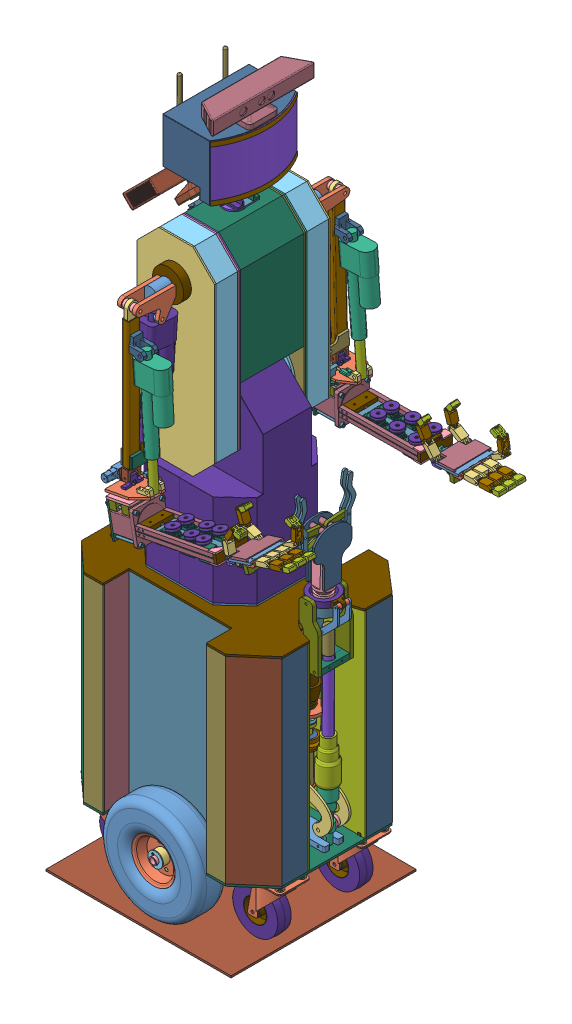
SolidWorks assembly sorbot, configuration По умолчанию. Lengths in mm. (continued)
Mates (geometry in assembly coordinates): (continued)
- Совпадение1215: coincident anti-aligned: plane of arm.rotate.p10-2 through (21.3669 899.2327 -464.7087) normal (0.012385 -0.99968 -0.022041); plane of arm.rotate-2/arm.rotate.p1-3 through (-38.6277 898.4966 -465.0367) normal (-0.012385 0.99968 0.022041)
- Заблокировать582: lock: unknown of ?; unknown of ?
- Концентричный657: concentric aligned: cylinder of arm.actuator100mm.p2-2 through (48.6447 928.0854 -396.9103) axis (0.005195 0.022106 -0.999742) radius 4; cylinder of arm.rotate.p7-3 through (48.824 928.8481 -431.4028) axis (0.005195 0.022106 -0.999742) radius 4
- Концентричный658: concentric aligned: cylinder of arm.rotate-2/SY85STH65-2808A-1 through (58.2497 849.7566 -423.1001) axis (-0.99991 -0.012267 -0.005467) radius 6; cylinder of arm.rotate.p9-3 through (59.2496 849.7688 -423.0946) axis (-0.99991 -0.012267 -0.005467) radius 6
- Концентричный659: concentric anti-aligned: cylinder of arm.rotate-2/SY85STH65-2808A-1 through (58.2497 849.7566 -423.1001) axis (-0.99991 -0.012267 -0.005467) radius 6; cylinder of arm.rotate.p9-4 through (29.2523 849.4008 -423.2587) axis (0.99991 0.012267 0.005467) radius 6
- Параллельность213: parallel anti-aligned: plane of arm.rotate.p9-3 through (59.4308 849.4876 -455.6083) normal (-0.012385 0.99968 0.022041); plane of arm.rotate.p9-4 through (29.4088 851.119 -455.7282) normal (0.012385 -0.99968 -0.022041)
- Совпадение1219: coincident anti-aligned: plane of lower.arm.p3-2 through (29.2723 850.5384 -429.474) normal (-0.012385 0.99968 0.022041); plane of arm.rotate.p9-4 through (29.4088 851.119 -455.7282) normal (0.012385 -0.99968 -0.022041)
- Совпадение1223: coincident aligned: plane of lower.arm.p2-8 through (29.6119 839.3549 -466.49) normal (-0.99991 -0.012267 -0.005467); plane of arm.rotate.p9-3 through (29.2197 837.6859 -391.0095) normal (-0.99991 -0.012267 -0.005467)
- Заблокировать583: lock: plane of ?; plane of ?
- Расстояние31: distance = 1 mm anti-aligned: plane of arm.rotate.p9-3 through (29.2197 837.6859 -391.0095) normal (-0.99991 -0.012267 -0.005467); plane of arm.rotate-2/SY85STH65-2808A-1 through (28.2524 849.3885 -423.2641) normal (0.99991 0.012267 0.005467)
- Совпадение1224: coincident aligned: plane of arm.rotate.p9-3 through (59.217 838.0539 -390.8455) normal (0.99991 0.012267 0.005467); plane of arm.rotate.p9-4 through (58.9445 860.0469 -390.3606) normal (0.99991 0.012267 0.005467)
- Заблокировать584: lock: unknown of ?; unknown of ?
- Заблокировать585: lock: unknown of ?; unknown of ?
- Совпадение1228: coincident anti-aligned: plane of arm.rotate.p11.mirr-1 through (-44.1127 919.5219 -423.5897) normal (-0.99991 -0.012267 -0.005467); plane of arm.elbow.rotate.p1-2 through (-44.401 942.7787 -423.0475) normal (0.99991 0.012267 0.005467)
- Концентричный660: concentric anti-aligned: cylinder of arm.rotate.p11.mirr-1 through (-44.4134 931.8709 -396.3113) axis (0.99991 0.012267 0.005467) radius 4.5; cylinder of arm.elbow.rotate.p1-2 through (-43.9134 931.877 -396.3085) axis (-0.99991 -0.012267 -0.005467) radius 4.5
- Заблокировать586: lock: unknown of ?; unknown of ?
- Совпадение1229: coincident anti-aligned: plane of arm.elbow.rotate.p4-2 through (-11.4253 903.8925 -422.2651) normal (0.012385 -0.99968 -0.022041); plane of arm.rotate.p10-2 through (21.2926 905.2308 -464.5765) normal (-0.012385 0.99968 0.022041)
- Заблокировать587: lock: unknown of ?; unknown of ?
- Заблокировать588: lock: unknown of ?; unknown of ?
- Концентричный661: concentric anti-aligned: cylinder of arm.elbow.rotate.p13-2 through (-43.5634 931.8813 -396.3066) axis (0.99991 0.012267 0.005467) radius 4.5; cylinder of arm.elbow.rotate.p14-2 through (-32.4144 932.0181 -396.2457) axis (-0.99991 -0.012267 -0.005467) radius 4.5
- Совпадение1230: coincident anti-aligned: plane of arm.rotate.p11.mirr-1 through (-42.1129 919.5464 -423.5788) normal (0.99991 0.012267 0.005467); plane of arm.elbow.rotate.p14-2 through (-42.4135 931.8954 -396.3003) normal (-0.99991 -0.012267 -0.005467)
- Совпадение1231: coincident anti-aligned: plane of arm.elbow.rotate.p1-2 through (-38.5639 931.9427 -396.2793) normal (0.99991 0.012267 0.005467); plane of arm.elbow.rotate.p5-2 through (-38.5639 931.9427 -396.2793) normal (-0.99991 -0.012267 -0.005467)
- Концентричный662: concentric anti-aligned: cylinder of arm.elbow.rotate.p13-2 through (-38.5639 931.9427 -396.2793) axis (0.99991 0.012267 0.005467) radius 2.5; cylinder of arm.elbow.rotate.p5-2 through (36.4293 932.8627 -395.8693) axis (-0.99991 -0.012267 -0.005467) radius 2.5
- Концентричный663: concentric anti-aligned: cylinder of arm.elbow.rotate.p5-2 through (36.4293 932.8627 -395.8693) axis (-0.99991 -0.012267 -0.005467) radius 2.5; cylinder of arm.elbow.rotate.p11-2 through (-1.4172 932.3984 -396.0762) axis (0.99991 0.012267 0.005467) radius 2.5
- Параллельность214: parallel aligned: plane of arm.rotate.p6-2 through (-44.267 912.5511 -379.7333) normal (0.012385 -0.99968 -0.022041); plane of arm.elbow.rotate.p11-2 through (-1.2154 908.6007 -379.597) normal (0.012385 -0.99968 -0.022041)
- Концентричный664: concentric aligned: cylinder of arm.elbow.rotate.p11-2 through (3.5157 928.5672 -375.1299) axis (0.012385 -0.99968 -0.022041) radius 2.5; cylinder of arm.elbow.rotate.p12-2 through (3.7634 908.5736 -375.5707) axis (0.012385 -0.99968 -0.022041) radius 2.5
- Совпадение1232: coincident anti-aligned: plane of arm.elbow.rotate.p11-2 through (-1.2154 908.6007 -379.597) normal (0.012385 -0.99968 -0.022041); plane of arm.elbow.rotate.p12-2 through (3.7634 908.5736 -375.5707) normal (-0.012385 0.99968 0.022041)
- Концентричный665: concentric aligned: cylinder of arm.rotate.p10-2 through (12.8933 903.4304 -387.6401) axis (0.012385 -0.99968 -0.022041) radius 2.5; cylinder of arm.elbow.rotate.p12-2 through (12.8249 908.9493 -387.5184) axis (0.012385 -0.99968 -0.022041) radius 2.5
- Параллельность215: parallel aligned: plane of arm.rotate.p6-2 through (-43.8997 920.4283 -464.5792) normal (-0.99991 -0.012267 -0.005467); plane of arm.rotate.p10-2 through (-43.6272 898.4353 -465.0641) normal (-0.99991 -0.012267 -0.005467)
- Заблокировать589: lock: unknown of ?; unknown of ?
- Заблокировать590: lock: unknown of ?; unknown of ?
- Совпадение1237: coincident anti-aligned: plane of palm.tilt.p1-2 through (73.3338 838.9402 -423.1109) normal (0.99991 0.012267 0.005467); plane of palm.drive.thread.fixture.p2-3 through (73.3338 838.9402 -423.1109) normal (-0.99991 -0.012267 -0.005467)
- Концентричный668: concentric aligned: cylinder of palm.tilt.p1-2 through (82.7829 839.0561 -423.0592) axis (-0.99991 -0.012267 -0.005467) radius 1.5; cylinder of palm.drive.thread.fixture.p2-3 through (88.3324 839.1242 -423.0288) axis (-0.99991 -0.012267 -0.005467) radius 1.5
- Концентричный669: concentric anti-aligned: cylinder of palm.drive.thread.fixture.p2-3 through (88.3324 839.1242 -423.0288) axis (0.99991 0.012267 0.005467) radius 2.5; cylinder of palm.lift.p2-3 through (243.2737 841.0251 -422.1817) axis (-0.99991 -0.012267 -0.005467) radius 2.5
- Концентричный670: concentric aligned: cylinder of palm.lift.p2-3 through (243.2737 841.0251 -422.1817) axis (-0.99991 -0.012267 -0.005467) radius 2.5; cylinder of palm.lift.drive.nut-2 through (168.3752 840.1062 -422.5912) axis (-0.99991 -0.012267 -0.005467) radius 2.5
- Заблокировать591: lock: unknown of ?; unknown of ?
- Заблокировать592: lock: unknown of ?; unknown of ?
- Концентричный672: concentric anti-aligned: cylinder of palm.lift.drive.nut-2 through (155.3763 839.9467 -422.6623) axis (0.99991 0.012267 0.005467) radius 4.5; cylinder of palm.lift.nut.fixture-3 through (165.3754 840.0694 -422.6076) axis (-0.99991 -0.012267 -0.005467) radius 4.5
- Концентричный673: concentric aligned: cylinder of palm.lift.drive.nut-2 through (155.3763 839.9467 -422.6623) axis (0.99991 0.012267 0.005467) radius 4.5; cylinder of palm.lift.nut.fixture-4 through (155.3763 839.9467 -422.6623) axis (0.99991 0.012267 0.005467) radius 4.5
- Параллельность217: parallel anti-aligned: plane of palm.lift.nut.fixture-4 through (165.2516 850.0662 -422.3872) normal (-0.012385 0.99968 0.022041); plane of lower.arm.p3-2 through (29.2971 848.5391 -429.5181) normal (0.012385 -0.99968 -0.022041)
- Параллельность218: parallel anti-aligned: plane of palm.lift.nut.fixture-3 through (155.2525 849.9435 -422.4419) normal (-0.012385 0.99968 0.022041); plane of lower.arm.p3-2 through (29.2971 848.5391 -429.5181) normal (0.012385 -0.99968 -0.022041)
- Совпадение1239: coincident aligned: plane of palm.lift.nut.fixture-3 through (165.5464 821.8541 -413.0069) normal (0.99991 0.012267 0.005467); plane of palm.lift.nut.fixture-4 through (165.6503 822.2962 -433.0018) normal (0.99991 0.012267 0.005467)
- Совпадение1240: coincident anti-aligned: plane of palm.lift.drive.nut-2 through (165.3754 840.0694 -422.6076) normal (-0.99991 -0.012267 -0.005467); plane of palm.lift.nut.fixture-3 through (165.5464 821.8541 -413.0069) normal (0.99991 0.012267 0.005467)
- Концентричный674: concentric anti-aligned: cylinder of palm.lift.nut.fixture-4 through (155.5366 827.0102 -422.9475) axis (0.99991 0.012267 0.005467) radius 2; cylinder of palm.lift.p4-2 through (270.9675 828.4263 -422.3163) axis (-0.99991 -0.012267 -0.005467) radius 2
- Заблокировать594: lock: unknown of ?; unknown of ?
- Заблокировать595: lock: unknown of ?; unknown of ?
- Концентричный675: concentric aligned: cylinder of palm.lift.fixture-2 through (263.588 847.6072 -437.0845) axis (-0.005195 -0.022106 0.999742) radius 3; cylinder of palm.lift.fixture.p2-2 through (263.588 847.6072 -437.0845) axis (-0.005195 -0.022106 0.999742) radius 3
- Совпадение1244: coincident anti-aligned: plane of palm.lift.fixture-2 through (256.1542 841.2966 -427.2601) normal (0.005195 0.022106 -0.999742); plane of palm.lift.fixture.p2-2 through (249.8978 852.5761 -427.0432) normal (-0.005195 -0.022106 0.999742)
- Концентричный676: concentric aligned: cylinder of palm.lift.fixture.p2-2 through (279.6623 840.7293 -421.9177) axis (-0.060104 0.997955 0.021755) radius 3; cylinder of m6.washer-4 through (279.464 844.0226 -421.8459) axis (-0.060104 0.997955 0.021755) radius 3.25
- Совпадение1245: coincident anti-aligned: plane of palm.lift.fixture.p2-2 through (270.5872 845.5238 -437.0942) normal (0.060104 -0.997955 -0.021755); plane of m6.washer-4 through (279.3618 845.7191 -421.8089) normal (-0.060104 0.997955 0.021755)
- Концентричный677: concentric anti-aligned: cylinder of palm.lift.fixture.p2-2 through (279.6623 840.7293 -421.9177) axis (-0.060104 0.997955 0.021755) radius 3; cylinder of m6.washer-5 through (278.7488 855.8982 -421.587) axis (0.060104 -0.997955 -0.021755) radius 3.25
- Совпадение1246: coincident anti-aligned: plane of m6.washer-5 through (278.8509 854.2017 -421.624) normal (0.060104 -0.997955 -0.021755); plane of palm.lift.fixture.p2-2 through (258.0981 853.2868 -436.9874) normal (-0.060104 0.997955 0.021755)
- Концентричный678: concentric aligned: cylinder of palm.fixture.p14-2 through (278.7488 855.8982 -421.587) axis (-0.060104 0.997955 0.021755) radius 3; cylinder of palm.lift.fixture.p2-2 through (279.6623 840.7293 -421.9177) axis (-0.060104 0.997955 0.021755) radius 3
- Совпадение1247: coincident anti-aligned: plane of palm.fixture.p14-2 through (314.7351 857.7336 -406.3556) normal (0.060104 -0.997955 -0.021755); plane of m6.washer-5 through (278.7488 855.8982 -421.587) normal (-0.060104 0.997955 0.021755)
- Концентричный680: concentric anti-aligned: cylinder of palm.fixture.p14-2 through (278.7488 855.8982 -421.587) axis (-0.060104 0.997955 0.021755) radius 3; cylinder of m6.washer-6 through (278.286 863.5825 -421.4195) axis (0.060104 -0.997955 -0.021755) radius 3.25
- Совпадение1248: coincident anti-aligned: plane of palm.fixture.p14-2 through (314.3745 863.7213 -406.2251) normal (-0.060104 0.997955 0.021755); plane of m6.washer-6 through (278.3881 861.886 -421.4565) normal (0.060104 -0.997955 -0.021755)
- Совпадение1249: coincident aligned: plane of palm.lift.p4-2 through (270.9675 828.4263 -422.3163) normal (0.99991 0.012267 0.005467); plane of palm.lift.fixture.p6-2 through (270.9675 828.4263 -422.3163) normal (0.99991 0.012267 0.005467)
- Концентричный681: concentric aligned: cylinder of palm.lift.p4-2 through (270.9675 828.4263 -422.3163) axis (-0.99991 -0.012267 -0.005467) radius 2; cylinder of palm.lift.fixture.p6-2 through (270.9675 828.4263 -422.3163) axis (-0.99991 -0.012267 -0.005467) radius 2
- Заблокировать596: lock: unknown of ?; unknown of ?
- Концентричный682: concentric anti-aligned: cylinder of palm.lift.on-palm.fixture-3 through (293.0416 835.5977 -409.1898) axis (0.005195 0.022106 -0.999742) radius 2; cylinder of palm.lift.fixture.p7-2 through (293.1196 835.9293 -424.1859) axis (-0.005195 -0.022106 0.999742) radius 2
- Совпадение1250: coincident anti-aligned: plane of palm.lift.fixture.p7-2 through (276.6855 828.4557 -420.4355) normal (-0.005195 -0.022106 0.999742); plane of palm.lift.on-palm.fixture-3 through (297.3768 831.3444 -420.2641) normal (0.005195 0.022106 -0.999742)
- Концентричный683: concentric aligned: cylinder of palm.lift.fixture.p6-2 through (276.7263 828.6292 -428.2835) axis (-0.005195 -0.022106 0.999742) radius 2; cylinder of palm.lift.fixture.p7-2 through (276.7063 828.5441 -424.4345) axis (-0.005195 -0.022106 0.999742) radius 2
- Заблокировать597: lock: unknown of ?; unknown of ?
- Заблокировать598: lock: unknown of ?; unknown of ?
- Концентричный684: concentric aligned: cylinder of palm.drive.thread.fixture.p2-4 through (319.6581 852.5389 -417.0976) axis (-0.005195 -0.022106 0.999742) radius 1.5; cylinder of palm.lift.p1-2 through (319.6293 852.4162 -411.549) axis (-0.005195 -0.022106 0.999742) radius 1.5
- Совпадение1257: coincident anti-aligned: plane of palm.lift.p1-2 through (319.5802 852.2073 -402.1015) normal (0.005195 0.022106 -0.999742); plane of palm.drive.thread.fixture.p2-4 through (319.5802 852.2073 -402.1015) normal (-0.005195 -0.022106 0.999742)
- Совпадение1258: coincident anti-aligned: plane of palm.drive.thread.fixture.p2-4 through (319.6581 852.5389 -417.0976) normal (0.005195 0.022106 -0.999742); plane of palm.tilit.p8-2 through (319.6581 852.5389 -417.0976) normal (-0.005195 -0.022106 0.999742)
- Концентричный685: concentric aligned: cylinder of palm.drive.thread.fixture.p2-4 through (319.6581 852.5389 -417.0976) axis (0.005195 0.022106 -0.999742) radius 2.5; cylinder of palm.tilit.p8-2 through (319.6581 852.5389 -417.0976) axis (0.005195 0.022106 -0.999742) radius 2.5
- Заблокировать599: lock: unknown of ?; unknown of ?
- Заблокировать600: lock: unknown of ?; unknown of ?
- Совпадение1264: coincident anti-aligned: plane of palm.tilit.p10-2 through (311.367 847.3638 -408.8344) normal (0.060104 -0.997955 -0.021755); plane of palm.tilit.p12-2 through (307.7969 847.4327 -421.8547) normal (-0.060104 0.997955 0.021755)
- Концентричный692: concentric anti-aligned: cylinder of palm.tilit.p10-2 through (307.7969 847.4327 -421.8547) axis (-0.060104 0.997955 0.021755) radius 2; cylinder of palm.tilit.p12-2 through (307.7969 847.4327 -421.8547) axis (0.060104 -0.997955 -0.021755) radius 2
- Концентричный693: concentric aligned: cylinder of palm.tilit.p8-2 through (319.6581 852.5389 -417.0976) axis (0.005195 0.022106 -0.999742) radius 2.5; cylinder of palm.tilit.p11-2 through (319.7594 852.9701 -436.6007) axis (0.005195 0.022106 -0.999742) radius 2.5
- Концентричный695: concentric anti-aligned: cylinder of palm.tilit.p12-2 through (309.6073 847.9757 -441.7652) axis (0.060104 -0.997955 -0.021755) radius 2; cylinder of palm.tilit.p11-2 through (309.5781 848.4611 -441.7546) axis (-0.060104 0.997955 0.021755) radius 2
- Параллельность220: parallel aligned: plane of arm.rotate.p10-2 through (21.2926 905.2308 -464.5765) normal (-0.012385 0.99968 0.022041); plane of arm.rotate.p9-4 through (29.2849 861.1158 -455.5078) normal (-0.012385 0.99968 0.022041)
- Заблокировать601: lock: unknown of ?; unknown of palm.drive.thread.fixture-2
- Концентричный696: concentric anti-aligned: cylinder of body.frame.p2-1 through (-12.4903 1112.7235 -136.5542) axis (0 1 0) radius 20; cylinder of SY57STH56-2804A-1 through (-12.4903 1435.8936 -136.5542) axis (0 -1 0) radius 19
- Совпадение1265: coincident anti-aligned: plane of body.frame.p2-1 through (33.4059 1434.2936 -222.3642) normal (0 -1 0); plane of SY57STH56-2804A-1 through (-35.4903 1434.2936 -159.5542) normal (0 1 0)
- Концентричный697: concentric aligned: cylinder of SY57STH56-2804A-1 through (-12.4903 1454.8936 -136.5542) axis (0 -1 0) radius 3.175; cylinder of head.tilt.p1-1 through (-12.4903 1454.7936 -136.5542) axis (0 -1 0) radius 3.175
- Концентричный698: concentric aligned: cylinder of SY57STH56-2804A-1 through (-12.4903 1454.8936 -136.5542) axis (0 -1 0) radius 3.175; cylinder of head.rotate.bearing-1 through (-12.4903 1444.7936 -136.5542) axis (0 -1 0) radius 8.5
- Совпадение1266: coincident anti-aligned: plane of SY57STH56-2804A-1 through (-12.4903 1435.8936 -136.5542) normal (0 1 0); plane of ? through (-12.4903 1435.8936 -136.5542) normal (0 -1 0)
- Совпадение1267: coincident anti-aligned: plane of SY57STH56-2804A-1 through (-12.4903 1435.8936 -136.5542) normal (0 1 0); plane of head.rotate.bearing.insert-1 through (-12.4903 1435.8936 -136.5542) normal (0 -1 0)
- Концентричный699: concentric aligned: cylinder of SY57STH56-2804A-1 through (-12.4903 1454.8936 -136.5542) axis (0 -1 0) radius 3.175; cylinder of ? through (-12.4903 1444.3936 -136.5542) axis (0 -1 0) radius 3.175
- Совпадение1268: coincident anti-aligned: plane of head.tilt.p1-1 through (-12.4903 1444.7936 -136.5542) normal (0 -1 0); plane of ? through (-12.4903 1444.7936 -136.5542) normal (0 1 0)
- Параллельность221: parallel anti-aligned: plane of body.frame.p2-1 through (33.4059 1436.2936 -222.3642) normal (0 1 0); plane of SY42STH47-1 through (-17.6903 1463.2936 -152.0542) normal (0 -1 0)
- Концентричный701: concentric aligned: cylinder of SY42STH47-1 through (-33.8403 1484.4436 -128.0542) axis (0 0 -1) radius 2.5; cylinder of head.tilt.p2-1 through (-33.8403 1484.4436 -134.5542) axis (0 0 -1) radius 2.5
- Заблокировать602: lock: unknown of ?; unknown of ?
- Концентричный705: concentric anti-aligned: cylinder of head.tilt.p1-1 through (-2.6766 1437.2936 -156.8012) axis (0 1 0) radius 2; cylinder of head.tilit.p4-1 through (-2.6766 1467.8044 -156.8012) axis (0 -1 0) radius 2
- Концентричный706: concentric anti-aligned: cylinder of head.tilt.p1-1 through (7.7567 1437.2936 -126.7405) axis (0 1 0) radius 2; cylinder of head.tilit.p4-2 through (7.7567 1467.8044 -126.7405) axis (0 -1 0) radius 2
- Концентричный707: concentric anti-aligned: cylinder of head.tilt.p1-1 through (-22.304 1437.2936 -116.3072) axis (0 1 0) radius 2; cylinder of head.tilit.p4-3 through (-22.304 1467.8044 -116.3072) axis (0 -1 0) radius 2
- Концентричный708: concentric anti-aligned: cylinder of head.tilt.p1-1 through (-32.7373 1437.2936 -146.3679) axis (0 1 0) radius 2; cylinder of head.tilit.p4-4 through (-32.7373 1467.8044 -146.3679) axis (0 -1 0) radius 2
- Совпадение1273: coincident anti-aligned: plane of head.tilt.p1-1 through (-12.4903 1441.2936 -136.5542) normal (0 1 0); plane of head.tilit.p4-4 through (-32.7373 1441.2936 -146.3679) normal (0 -1 0)
- Совпадение1274: coincident anti-aligned: plane of head.tilt.p1-1 through (-12.4903 1441.2936 -136.5542) normal (0 1 0); plane of head.tilit.p4-3 through (-22.304 1441.2936 -116.3072) normal (0 -1 0)
- Совпадение1275: coincident anti-aligned: plane of head.tilt.p1-1 through (-12.4903 1441.2936 -136.5542) normal (0 1 0); plane of head.tilit.p4-1 through (-2.6766 1441.2936 -156.8012) normal (0 -1 0)
- Совпадение1276: coincident anti-aligned: plane of head.tilt.p1-1 through (-12.4903 1441.2936 -136.5542) normal (0 1 0); plane of head.tilit.p4-2 through (7.7567 1441.2936 -126.7405) normal (0 -1 0)
- Концентричный709: concentric aligned: cylinder of SY57STH56-2804A-1 through (-12.4903 1454.8936 -136.5542) axis (0 -1 0) radius 3.175; cylinder of head.p1-1 through (-12.4903 1458.2936 -136.5542) axis (0 -1 0) radius 3.175
- Совпадение1277: coincident anti-aligned: plane of head.tilt.p1-1 through (-12.4903 1454.7936 -136.5542) normal (0 1 0); plane of head.p1-1 through (30.0097 1454.7936 -164.0542) normal (0 -1 0)
- Совпадение1278: coincident anti-aligned: plane of head.p1-1 through (30.0097 1458.2936 -164.0542) normal (0 1 0); plane of head.tilit.p5-1 through (30.0097 1458.2936 -148.0542) normal (0 -1 0)
- Совпадение1279: coincident anti-aligned: plane of SY42STH47-1 through (-17.6903 1463.2936 -152.0542) normal (0 -1 0); plane of head.tilit.p5-1 through (30.0097 1463.2936 -152.0542) normal (0 1 0)
- Совпадение1280: coincident aligned: plane of SY42STH47-1 through (-54.9903 1468.2936 -152.0542) normal (-1 0 0); plane of head.tilit.p5-1 through (-54.9903 1505.5936 -152.0542) normal (-1 0 0)
- Совпадение1281: coincident anti-aligned: plane of SY42STH47-1 through (-54.9903 1463.2936 -152.0542) normal (0 0 1); plane of head.tilit.p5-1 through (30.0097 1463.2936 -152.0542) normal (0 0 -1)
- Совпадение1283: coincident aligned: plane of head.p1-1 through (-54.9903 1458.2936 -105.9254) normal (-1 0 0); plane of head.tilit.p5-1 through (-54.9903 1505.5936 -152.0542) normal (-1 0 0)
- Заблокировать606: lock: unknown of ?; unknown of ?
- Параллельность222: parallel aligned: plane of body.frame.p2-1 through (92.5097 1112.7235 -222.3642) normal (1 0 0); plane of head.p1-1 through (30.0097 1458.2936 -105.9254) normal (1 0 0)
- Расстояние32: distance = 0.4 mm aligned: plane of head.tilt.p8-1 through (-4.1768 1486.067 -134.1542) normal (0 0 1); plane of head.tilt.p2-1 through (-33.8403 1484.4436 -134.5542) normal (0 0 1)
- Концентричный711: concentric anti-aligned: cylinder of head.tilt.p8-1 through (-4.1768 1486.067 -139.0542) axis (0 0 1) radius 3; cylinder of head.tilt.p9-1 through (-4.1768 1486.067 -112.7074) axis (0 0 -1) radius 3
- Совпадение1286: coincident anti-aligned: plane of head.p1-1 through (30.0097 1458.2936 -164.0542) normal (0 1 0); plane of head.tilit.p5.m-1 through (-54.9903 1458.2936 -121.9254) normal (0 -1 0)
- Совпадение1287: coincident aligned: plane of head.p1-1 through (-54.9903 1458.2936 -105.9254) normal (-1 0 0); plane of head.tilit.p5.m-1 through (-54.9903 1505.5936 -117.9254) normal (-1 0 0)
- Концентричный713: concentric anti-aligned: cylinder of head.tilt.p8-1 through (-4.1768 1486.067 -141.0542) axis (0 0 1) radius 4.85; cylinder of head.tilt.p10-1 through (-4.1768 1486.067 -138.0542) axis (0 0 -1) radius 4.85
- Совпадение1288: coincident anti-aligned: plane of head.tilt.p8-1 through (-4.1768 1486.067 -138.0542) normal (0 0 -1); plane of head.tilt.p10-1 through (-4.1768 1486.067 -138.0542) normal (0 0 1)
- Концентричный714: concentric anti-aligned: cylinder of head.tilt.p8-1 through (-4.1768 1486.067 -132.1542) axis (0 0 -1) radius 4.85; cylinder of head.tilt.p10-2 through (-4.1768 1486.067 -135.1542) axis (0 0 1) radius 4.85
- Совпадение1289: coincident anti-aligned: plane of head.tilt.p8-1 through (-4.1768 1486.067 -135.1542) normal (0 0 1); plane of head.tilt.p10-2 through (-4.1768 1486.067 -135.1542) normal (0 0 -1)
- Концентричный715: concentric anti-aligned: cylinder of head.tilt.p10-2 through (-4.1768 1486.067 -135.1542) axis (0 0 1) radius 4.85; cylinder of head.tilit.p11-1 through (-4.1768 1486.067 -128.1542) axis (0 0 -1) radius 1
- Совпадение1290: coincident anti-aligned: plane of head.tilt.p10-2 through (-4.1768 1486.067 -131.6542) normal (0 0 1); plane of head.tilit.p11-1 through (-6.8677 1566.0217 -131.6542) normal (0 0 -1)
- Концентричный716: concentric aligned: cylinder of head.tilt.p10-1 through (-4.1768 1486.067 -138.0542) axis (0 0 -1) radius 4.85; cylinder of head.tilit.p11-2 through (-4.1768 1486.067 -141.5542) axis (0 0 -1) radius 1
- Совпадение1291: coincident anti-aligned: plane of head.tilt.p10-1 through (-4.1768 1486.067 -141.5542) normal (0 0 -1); plane of head.tilit.p11-2 through (-6.8677 1566.0217 -141.5542) normal (0 0 1)
- Совпадение1292: coincident aligned: plane of head.tilit.p11-1 through (8.1238 1566.5263 -128.1542) normal (0.99746 0.071224 0); plane of head.tilit.p11-2 through (8.1238 1566.5263 -141.5542) normal (0.99746 0.071224 0)
- Заблокировать608: lock: unknown of ?; unknown of ?
- Заблокировать609: lock: unknown of ?; unknown of ?
- Заблокировать610: lock: unknown of ?; unknown of ?
- Заблокировать611: lock: unknown of ?; unknown of ?
- Концентричный718: concentric anti-aligned: cylinder of head.tilit.p5-1 through (-4.1768 1486.067 -164.0542) axis (0 0 1) radius 3; cylinder of head.tilt.p9-1 through (-4.1768 1486.067 -112.7074) axis (0 0 -1) radius 3
- Концентричный720: concentric aligned: cylinder of head.tilt.p9-1 through (-4.1768 1486.067 -112.7074) axis (0 0 -1) radius 3; cylinder of head.tilt.p12-2 through (-4.1768 1486.067 -145.0542) axis (0 0 -1) radius 3
- Совпадение1294: coincident anti-aligned: plane of head.tilit.p5-1 through (30.0097 1458.2936 -148.0542) normal (0 0 1); plane of head.tilt.p12-2 through (-4.1768 1486.067 -148.0542) normal (0 0 -1)
- Концентричный721: concentric anti-aligned: cylinder of head.tilit.p11-1 through (5.0356 1476.8947 -128.1542) axis (0 0 -1) radius 2; cylinder of m4.nut-5 through (5.0356 1476.8947 -128.1542) axis (0 0 1) radius 2
- Концентричный723: concentric anti-aligned: cylinder of head.tilit.p11-1 through (-4.1485 1473.067 -128.1542) axis (0 0 -1) radius 2; cylinder of m4.nut-6 through (-4.1485 1473.067 -128.1542) axis (0 0 1) radius 2
- Концентричный724: concentric anti-aligned: cylinder of head.tilit.p11-1 through (-13.3492 1476.8546 -128.1542) axis (0 0 -1) radius 2; cylinder of m4.nut-7 through (-13.3492 1476.8546 -128.1542) axis (0 0 1) radius 2
- Концентричный725: concentric anti-aligned: cylinder of head.tilit.p11-1 through (4.9956 1495.2794 -128.1542) axis (0 0 -1) radius 2; cylinder of m4.nut-3 through (4.9956 1495.2794 -128.1542) axis (0 0 1) radius 2
- Концентричный726: concentric anti-aligned: cylinder of head.tilit.p11-1 through (-4.2051 1499.067 -128.1542) axis (0 0 -1) radius 2; cylinder of m4.nut-4 through (-4.2051 1499.067 -128.1542) axis (0 0 1) radius 2
- Концентричный727: concentric anti-aligned: cylinder of head.tilit.p11-1 through (-13.3892 1495.2394 -128.1542) axis (0 0 -1) radius 2; cylinder of m4.nut-8 through (-13.3892 1495.2394 -128.1542) axis (0 0 1) radius 2
- Совпадение1295: coincident anti-aligned: plane of head.tilit.p11-1 through (-6.8677 1566.0217 -128.1542) normal (0 0 1); plane of m4.nut-8 through (-13.3892 1499.2 -128.1542) normal (0 0 -1)
- Совпадение1296: coincident anti-aligned: plane of head.tilit.p11-1 through (-6.8677 1566.0217 -128.1542) normal (0 0 1); plane of m4.nut-4 through (-4.2051 1503.0276 -128.1542) normal (0 0 -1)
- Совпадение1297: coincident anti-aligned: plane of head.tilit.p11-1 through (-6.8677 1566.0217 -128.1542) normal (0 0 1); plane of m4.nut-3 through (4.9956 1499.24 -128.1542) normal (0 0 -1)
- Совпадение1298: coincident anti-aligned: plane of head.tilit.p11-1 through (-6.8677 1566.0217 -128.1542) normal (0 0 1); plane of m4.nut-7 through (-13.3492 1480.8153 -128.1542) normal (0 0 -1)
- Совпадение1299: coincident anti-aligned: plane of head.tilit.p11-1 through (-6.8677 1566.0217 -128.1542) normal (0 0 1); plane of m4.nut-6 through (-4.1485 1477.0277 -128.1542) normal (0 0 -1)
- Совпадение1300: coincident anti-aligned: plane of head.tilit.p11-1 through (-6.8677 1566.0217 -128.1542) normal (0 0 1); plane of m4.nut-5 through (5.0356 1480.8553 -128.1542) normal (0 0 -1)
- Концентричный728: concentric aligned: cylinder of head.tilt.p9-1 through (-4.1768 1486.067 -112.7074) axis (0 0 -1) radius 3; cylinder of m6.washer-7 through (-4.1768 1486.067 -116.2254) axis (0 0 -1) radius 3.25
- Совпадение1301: coincident anti-aligned: plane of head.tilit.p5.m-1 through (-54.9903 1463.2936 -117.9254) normal (0 0 1); plane of m6.washer-7 through (-4.1768 1486.067 -117.9254) normal (0 0 -1)
- Концентричный729: concentric anti-aligned: cylinder of head.tilt.p9-1 through (-4.1768 1486.067 -112.7074) axis (0 0 -1) radius 3; cylinder of m6.washer-8 through (-4.1768 1486.067 -153.7542) axis (0 0 1) radius 3.25
- Совпадение1302: coincident anti-aligned: plane of head.tilit.p5-1 through (30.0097 1463.2936 -152.0542) normal (0 0 -1); plane of m6.washer-8 through (-4.1768 1486.067 -152.0542) normal (0 0 1)
- Заблокировать612: lock: unknown of ?; unknown of ?
- Концентричный730: concentric aligned: cylinder of head.tilt.p9-1 through (-4.1768 1486.067 -112.7074) axis (0 0 -1) radius 3; cylinder of head.tilt.p12.m-1 through (-4.1768 1486.067 -121.6542) axis (0 0 -1) radius 3
- Совпадение1303: coincident anti-aligned: plane of head.tilit.p11-1 through (-6.8677 1566.0217 -128.1542) normal (0 0 1); plane of head.tilt.p12.m-1 through (-4.1768 1486.067 -128.1542) normal (0 0 -1)
- Совпадение1304: coincident aligned: plane of head.p1-1 through (-54.9903 1458.2936 -105.9254) normal (0 0 1); plane of head.tilit.p5.m-1 through (-54.9903 1463.2936 -105.9254) normal (0 0 1)
- Совпадение1305: coincident aligned: plane of head.p1-1 through (-54.9903 1458.2936 -164.0542) normal (0 0 -1); plane of head.tilit.p5-1 through (30.0097 1463.2936 -164.0542) normal (0 0 -1)
- Концентричный731: concentric anti-aligned: cylinder of head.tilit.p11-1 through (-6.8677 1566.0217 -128.1542) axis (0 0 -1) radius 15; cylinder of head.tilt.p13-1 through (-6.8677 1566.0217 -183.9806) axis (0 0 1) radius 15
- Совпадение1306: coincident anti-aligned: plane of head.tilit.p11-1 through (-6.8677 1566.0217 -131.6542) normal (0 0 -1); plane of head.tilt.p13-1 through (-6.8677 1566.0217 -131.6542) normal (0 0 1)
- Концентричный732: concentric aligned: cylinder of head.p3-1 through (-6.8677 1566.0217 -114.1542) axis (0 0 -1) radius 15.102; cylinder of head.tilit.p11-1 through (-6.8677 1566.0217 -128.1542) axis (0 0 -1) radius 15
- Совпадение1307: coincident anti-aligned: plane of head.tilit.p11-1 through (-6.8677 1566.0217 -128.1542) normal (0 0 1); plane of head.p3-1 through (-21.8677 1551.1571 -128.1542) normal (0 0 -1)
- Концентричный733: concentric anti-aligned: cylinder of head.tilit.p11-2 through (-6.8677 1566.0217 -141.5542) axis (0 0 -1) radius 15; cylinder of head.p3-2 through (-6.8677 1566.0217 -159.0542) axis (0 0 1) radius 15.102
- Совпадение1308: coincident anti-aligned: plane of head.tilit.p11-2 through (-6.8677 1566.0217 -145.0542) normal (0 0 -1); plane of head.p3-2 through (8.1323 1551.1571 -145.0542) normal (0 0 1)
- Совпадение1309: coincident anti-aligned: plane of head.tilit.p11-2 through (-6.8677 1566.0217 -145.0542) normal (0 0 -1); plane of head.p2-1 through (-23.5768 1549.1571 -145.0542) normal (0 0 1)
- Совпадение1311: coincident anti-aligned: plane of head.p3-1 through (-21.8677 1549.1571 -126.1542) normal (0 -1 0); plane of head.p2-1 through (38.3461 1549.1571 -213.999) normal (0 1 0)
- Совпадение1312: coincident: plane of head.tilit.p11-1 through (8.1238 1566.5263 -128.1542) normal (0.99746 0.071224 0); line of head.p2-1 through (9.3641 1549.1571 -128.0542) axis (0 0 -1)
- Заблокировать614: lock: unknown of ?; unknown of ?
- Заблокировать615: lock: unknown of ?; unknown of ?
- Заблокировать616: lock: unknown of ?; unknown of ?
- Заблокировать617: lock: unknown of ?; unknown of ?
- Параллельность225: parallel aligned: plane of ? through (39.4049 1529.1684 -213.999) normal (0 1 0); plane of ? through (-136.7624 1647.1684 -136.5542) normal (0 1 0)
- Расстояние33: distance = 30 mm aligned: plane of ? through (39.4049 1527.1684 -213.999) normal (0 -1 0); plane of ? through (-136.7624 1497.1684 -136.5542) normal (0 -1 0)
- Концентричный735: concentric aligned: cylinder of head.p2-1 through (23.3461 1547.1571 -198.999) axis (0 1 0) radius 5; circle of logitech.sphere.af-2
- Концентричный736: concentric aligned: cylinder of head.p2-1 through (23.3461 1547.1571 -74.1093) axis (0 1 0) radius 5; circle of logitech.sphere.af-1
- Касательный55: tangent aligned: unknown of ?; cylinder of ? through (-136.7624 1647.1684 -136.5542) axis (0 -1 0) radius 211.7321
- Касательный56: tangent aligned: unknown of ?; cylinder of ? through (-136.7624 1647.1684 -136.5542) axis (0 -1 0) radius 211.7321
- Расстояние34: distance = 38.4 mm: plane of ? through (-26.0264 1529.1684 -59.1093) normal (0 0 1); line of ? through (40.4676 1647.1684 -20.7093) axis (0 -1 0)
- Заблокировать618: lock: unknown of ?; unknown of ?
- Параллельность226: parallel aligned: plane of head.p1-1 through (30.0097 1458.2936 -105.9254) normal (1 0 0); plane of head.p2-1 through (38.3461 1549.1571 -59.1093) normal (1 0 0)
- Концентричный737: concentric anti-aligned: cylinder of head.glass-1 through (-137.8212 1667.1571 -136.5542) axis (0 -1 0) radius 214.7321; cylinder of head.glass.fixture-1 through (-137.8213 1517.1571 -136.5542) axis (0 1 0) radius 214.7321
- Концентричный738: concentric anti-aligned: cylinder of head.glass-1 through (-137.8212 1667.1571 -136.5542) axis (0 -1 0) radius 214.7321; cylinder of head.glass.fixture-2 through (-137.8212 1655.1571 -136.5542) axis (0 1 0) radius 214.7321
- Совпадение1313: coincident aligned: plane of head.glass-1 through (-137.8212 1667.1571 -136.5542) normal (0 1 0); plane of head.glass.fixture-2 through (-137.8212 1667.1571 -136.5542) normal (0 1 0)
- Совпадение1314: coincident aligned: plane of head.glass-1 through (41.9199 1667.1571 -19.0679) normal (-0.547129 0 0.837048); plane of head.glass.fixture-2 through (41.9199 1655.1571 -19.0679) normal (-0.547129 0 0.837048)
- Совпадение1315: coincident aligned: plane of head.glass-1 through (-137.8213 1517.1571 -136.5542) normal (0 -1 0); plane of head.glass.fixture-1 through (-137.8213 1517.1571 -136.5542) normal (0 -1 0)
- Совпадение1316: coincident aligned: plane of head.glass-1 through (41.9199 1667.1571 -19.0679) normal (-0.547129 0 0.837048); plane of head.glass.fixture-1 through (41.9199 1517.1571 -19.0679) normal (-0.547129 0 0.837048)
- Концентричный739: concentric anti-aligned: cylinder of head.glass-1 through (-137.8212 1667.1571 -136.5542) axis (0 -1 0) radius 211.7321; cylinder of head.p4-1 through (-137.8213 1517.1571 -136.5542) axis (0 1 0) radius 211.73
- Совпадение1317: coincident aligned: plane of head.glass-1 through (-137.8213 1517.1571 -136.5542) normal (0 -1 0); plane of head.p4-1 through (-137.8213 1517.1571 -136.5542) normal (0 -1 0)
- Заблокировать619: lock: unknown of head.p2-1; unknown of head.p4-1
- Совпадение1319: coincident anti-aligned: plane of head.p4-1 through (-84.6104 1578.1571 -252.4244) normal (-1 0 0); plane of ant-3 through (-84.6104 1643.7707 -74.539) normal (1 0 0)
- Совпадение1321: coincident anti-aligned: plane of head.p4-1 through (-84.6104 1578.1571 -252.4244) normal (-1 0 0); plane of ant-2 through (-84.6104 1643.7707 -198.1028) normal (1 0 0)
- Параллельность229: parallel aligned: plane of head.p4-1 through (39.3896 1666.1571 -253.5244) normal (0 0 -1); plane of ant-2 through (-96.1462 1641.4075 -199.6028) normal (0 0 -1)
- Параллельность230: parallel aligned: plane of head.p4-1 through (39.3896 1666.1571 -253.5244) normal (0 0 -1); plane of ant-3 through (-96.1462 1641.4075 -76.039) normal (0 0 -1)
- Заблокировать622: lock: unknown of ?; unknown of head.p4-1
- Заблокировать623: lock: unknown of head.p4-1; unknown of ant-2
- Параллельность231: parallel: plane of kinect-black-1 through (-305.9508 1681.1571 -96.5839) normal (0 0 1); plane of head.p4-1 through (-86.6104 1667.1571 -19.5839) normal (0 0 1)
- Совпадение1322: coincident: plane of head.p4-1 through (-137.3095 1668.1571 -136.5542) normal (0 1 0); plane of ? through (-305.9508 1668.1571 -166.5839) normal (0 -1 0)
- Расстояние35: distance = 77 mm aligned: plane of ? through (-305.9508 1681.1571 -96.5839) normal (0 0 1); plane of head.p4-1 through (-86.6104 1667.1571 -19.5839) normal (0 0 1)
- Заблокировать624: lock: unknown of head.p4-1; unknown of kinect-black-1
- Концентричный740: concentric anti-aligned: cylinder of S03T STD GWS Servo-1 through (-96.6103 1417.7008 -132.5396) axis (0.707107 -0.707107 0) radius 2.5; cylinder of back-kinect-servo-1 through (-95.3375 1416.428 -132.5396) axis (-0.707107 0.707107 0) radius 2.5
- Расстояние38: distance = 6.7 mm anti-aligned: plane of S03T STD GWS Servo-1 through (-85.537 1420.9959 -100.8996) normal (-0.707107 0.707107 0); plane of back-kinect-servo-1 through (-97.4588 1418.5493 -132.5396) normal (0.707107 -0.707107 0)
- Совпадение1323: coincident anti-aligned: plane of body.frame.p2-1 through (-58.3864 1436.2936 -222.3642) normal (-0.707107 0.707107 0); plane of S03T STD GWS Servo-1 through (-118.2623 1376.4177 -121.2196) normal (0.707107 -0.707107 0)
- Расстояние39: distance = 33.25 mm: line of body.frame.p2-1 through (-117.4903 1377.1897 -222.3642) axis (0 0 1); plane of S03T STD GWS Servo-1 through (-93.979 1400.701 -141.5396) normal (-0.707107 -0.707107 0)
- Расстояние42: distance = 74.5 mm: line of body.frame.p2-1 through (-58.3864 1436.2936 -222.3642) axis (-0.707107 -0.707107 0); plane of S03T STD GWS Servo-1 through (-119.9461 1378.1015 -147.8642) normal (0 0 -1)
- Совпадение1324: coincident anti-aligned: plane of kinect-1 through (-84.5541 1437.4644 -102.5396) normal (0.707107 -0.707107 0); plane of back-kinect-fixture-1 through (-116.3739 1405.6446 -102.5396) normal (-0.707107 0.707107 0)
- Совпадение1325: coincident aligned: plane of kinect-1 through (-93.7465 1446.6568 -172.5396) normal (0 0 -1); plane of back-kinect-fixture-1 through (-116.3739 1405.6446 -172.5396) normal (0 0 -1)
- Совпадение1326: coincident aligned: plane of kinect-1 through (-86.6754 1453.7278 -102.5396) normal (0.707107 0.707107 0); plane of back-kinect-fixture-1 through (-77.483 1444.5355 -102.5396) normal (0.707107 0.707107 0)
- Концентричный743: concentric aligned: cylinder of back-kinect-servo-1 through (-99.0498 1420.1403 -132.5396) axis (0.707107 -0.707107 0) radius 22.25; cylinder of back-kinect-fixture-1 through (-100.464 1421.5545 -132.5396) axis (0.707107 -0.707107 0) radius 5
- Совпадение1327: coincident anti-aligned: plane of back-kinect-servo-1 through (-99.0498 1420.1403 -132.5396) normal (-0.707107 0.707107 0); plane of back-kinect-fixture-1 through (-114.9597 1404.2304 -102.5396) normal (0.707107 -0.707107 0)
- Заблокировать625: lock: unknown of back-kinect-servo-1; unknown of back-kinect-fixture-1
- Параллельность232: parallel aligned: plane of wall11-1 through (-275.9003 882.565 11.9312) normal (-1 0 0); plane of turret.table-1 through (-172.5648 612.7934 -218.9555) normal (-1 0 0)
- Совпадение1329: coincident aligned: plane of body_pivot-2 through (-90.0648 982.0246 -71.9555) normal (0 0 1); plane of body.cover-1 through (-20.0648 1083.2934 -71.9555) normal (0 0 1)
- Расстояние43: distance = 470 mm anti-aligned: plane of body.cover-1 through (49.9352 1082.7934 -201.9555) normal (0 -1 0); plane of turret.table-1 through (-20.0648 612.7934 -360.2969) normal (0 1 0)
- Совпадение1330: coincident aligned: plane of body.cover-1 through (70.7211 612.7934 -276.3258) normal (0 0 -1); plane of body.cover-2 through (-110.834 860.7397 -276.3258) normal (0 0 -1)
- Совпадение1331: coincident aligned: plane of body.cover-1 through (49.9352 1083.2934 -201.9555) normal (0 1 0); plane of body.cover-2 through (-90.0648 1083.2934 -71.9735) normal (0 1 0)
- Совпадение1332: coincident anti-aligned: plane of body.cover-1 through (-20.0648 1083.2934 -71.9555) normal (-1 0 0); plane of body.cover-2 through (-20.0648 1083.2934 -201.9735) normal (1 0 0)
- Эскиз5: unknown: axis of sproket.initial-1 through (53.2168 119.2767 -271.5001) axis (0 0 -1); line of sprocket-1 through (-6.6918 11.9368 -268.3681) axis (0 0 -1); plane of sproket.initial-1 through (64.3825 152.5534 -271.5001) normal (0 0 -1)
- Эскиз6: unknown: line of turret-1/turret-p1-1 through (-20.0648 603.2934 -136.9555) axis (0 -1 0); unknown of man1-2/man1.p40-6; unknown of wall2-1; unknown of turret.table.cap-1; unknown of body_tilt_drive_frame_cap-1; unknown of body_tilt_drive_frame_cap-1; unknown of body_tilt_drive_frame_cap-1; unknown of body_tilt_drive_frame_cap-1; unknown of body_tilt_drive_frame_cap-1; unknown of lower.arm.p2-1; unknown of palm.p3-1; unknown of palm.p3.m-1; unknown of palm.p3-1; unknown of shoulder.axis-1; unknown of shoulder.axis-1; unknown of body.tilit.nut.housing-1; unknown of ?; unknown of ?; unknown of body_pivot_fixture-1; unknown of body_tilt_axis_clamp-1; unknown of body.tilit.planetary.drive.fixture.p5-1; unknown of body.tilit.planetary.drive.fixture.p5-1; unknown of body.tilit.planetary.drive.fixture.p5-1; unknown of body.tilit.planetary.drive.fixture.p5-1; unknown of shoulder.p6-2; unknown of shoulder.p6-2; unknown of lower.arm.p2-1; unknown of lower.arm.p2-1; unknown of lower.arm.p2-1; unknown of lower.arm.p2-1; unknown of lower.arm.p2-3; unknown of lower.arm.p2-3; unknown of lower.arm.p2-3; unknown of lower.arm.p2-3; unknown of arm.elbow.rotate.p1-1; unknown of arm.elbow.rotate.p1-1; unknown of arm.elbow.rotate.p1-1; unknown of arm.elbow.rotate.p1-1; unknown of arm.rotate.p7-2; unknown of arm.rotate.p7-2; unknown of arm.rotate.p7-2; unknown of palm.lift.drive.nut-1; unknown of palm.lift.nut.fixture-1; unknown of palm.lift.nut.fixture-2; unknown of palm.fixture.p14-1; unknown of palm.fixture.p14-1; unknown of palm.p1-3; unknown of palm.drive.thread.fixture.p2-2; unknown of palm.lift.on-palm.fixture-2; unknown of palm.lift.on-palm.fixture-2; unknown of palm.lift.on-palm.fixture-2; unknown of palm.lift.on-palm.fixture-2; unknown of palm.lift.on-palm.fixture-2; unknown of palm.lift.on-palm.fixture-2; unknown of arm.rotate.p7-2; unknown of arm.rotate.p7-2; unknown of SY57STH56-2804A-1; unknown of SY57STH56-2804A-1; unknown of head.tilt.p1-1; unknown of head.tilt.p1-1; unknown of head.tilt.p1-1; unknown of head.tilit.p4-1; unknown of head.tilit.p4-4; unknown of head.tilit.p4-2; unknown of head.tilit.p4-3; unknown of head.tilt.p1-1; unknown of head.tilt.p1-1; unknown of head.tilit.p4-1; unknown of head.tilit.p4-4; unknown of head.tilit.p4-2; unknown of head.tilit.p4-3; unknown of head.tilt.p8-1; unknown of head.tilt.p8-1; unknown of head.tilt.p8-1; unknown of head.tilt.p8-1; unknown of head.tilt.p8-1; unknown of head.tilt.p8-1; unknown of head.tilt.p8-1; unknown of head.tilt.p8-1; unknown of head.tilt.p8-1; unknown of head.tilt.p8-1; unknown of head.tilt.p8-1; unknown of head.tilt.p8-1; unknown of head.tilt.p10-2; unknown of head.tilt.p10-2; unknown of head.tilt.p10-2; unknown of head.tilt.p10-2; unknown of head.tilt.p10-2; unknown of head.tilt.p10-2; unknown of head.tilt.p10-2; unknown of head.tilt.p10-2; unknown of head.tilt.p10-2; unknown of head.tilt.p10-2; unknown of head.tilt.p10-2; unknown of head.tilt.p10-2; unknown of head.tilt.p9-1; unknown of head.tilt.p9-1; unknown of head.tilt.p9-1; unknown of head.tilt.p9-1; unknown of turret.table-1; unknown of turret.table-1; unknown of turret.table-1; unknown of turret.table-1; unknown of turret.table-1; unknown of turret.table-1; unknown of turret.table-1
